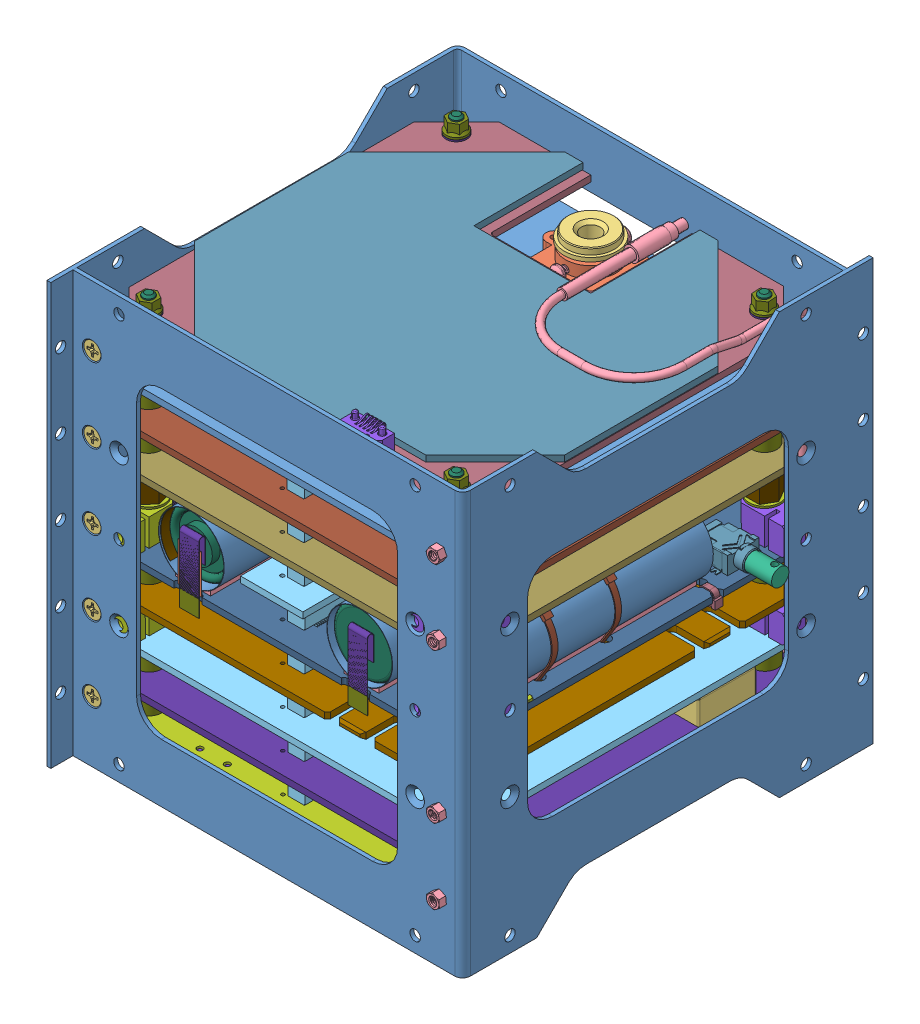
SolidWorks assembly FOX_FrameAssembly, configuration Default. Lengths in mm. (continued)
Components (placement in the parent): (continued)
- PCB-Stack-1: PCB-Stack [Default] at (24.8941 -34.8331 -20.5973) x (1 0 0) z (0 0.999997 0.002368) size (103.5 98 104.43) (continued)
  - PCB-Stack.iam-1: PCB-Stack.iam [Default] at origin size (103.5 98 104.43) (continued)
    - PCB_Exp4.iam-1: PCB_Exp4.iam [Default] at (0 0 87.6375) size (95 95 12.37) (continued)
      - Tant_Exp4_top.ipt-1: Tant_Exp4_top.ipt [Default] at (0 0 2.5749) size (95 95 1.57)
    - threaded_rod.ipt-1: threaded_rod.ipt [Default] at (-39.5 -39.5 44.6125) size (2.84 2.84 98)
    - threaded_rod.ipt-2: threaded_rod.ipt [Default] at (-39.5 39.5 44.6125) size (2.84 2.84 98)
    - threaded_rod.ipt-3: threaded_rod.ipt [Default] at (39.5 -39.5 44.6125) size (2.84 2.84 98)
    - threaded_rod.ipt-4: threaded_rod.ipt [Default] at (39.5 39.5 44.6125) size (2.84 2.84 98)
    - MS21043-04.ipt-1: MS21043-04.ipt [Default] at (-39.5 -39.5 -0.4064) x (1 0 0) z (0 0 -1) size (5.23 5.23 3.17)
    - MS21043-04.ipt-2: MS21043-04.ipt [Default] at (-39.5 39.5 -0.4064) x (1 0 0) z (0 0 -1) size (5.23 5.23 3.17)
    - MS21043-04.ipt-3: MS21043-04.ipt [Default] at (39.5 39.5 -0.4064) x (1 0 0) z (0 0 -1) size (5.23 5.23 3.17)
    - MS21043-04.ipt-4: MS21043-04.ipt [Default] at (39.5 -39.5 -0.4064) x (1 0 0) z (0 0 -1) size (5.23 5.23 3.17)
    - MS21043-04.ipt-5: MS21043-04.ipt [Default] at (-39.5 -39.5 89.6314) size (5.23 5.23 3.17)
    - MS21043-04.ipt-6: MS21043-04.ipt [Default] at (-39.5 39.5 89.6314) size (5.23 5.23 3.17)
    - MS21043-04.ipt-7: MS21043-04.ipt [Default] at (39.5 39.5 89.6314) x (0.997878 0.065108 0) z (0 0 1) size (5.23 5.23 3.17)
    - MS21043-04.ipt-8: MS21043-04.ipt [Default] at (39.5 -39.5 89.6314) size (5.23 5.23 3.17)
    - NAS620-4L.ipt-1: NAS620-4L.ipt [Default] at (-39.5 -39.5 -0.2032) x (1 0 0) z (0 0 -1) size (5.31 5.31 0.41)
    - NAS620-4L.ipt-2: NAS620-4L.ipt [Default] at (-39.5 39.5 -0.2032) x (1 0 0) z (0 0 -1) size (5.31 5.31 0.41)
    - NAS620-4L.ipt-3: NAS620-4L.ipt [Default] at (39.5 39.5 -0.2032) x (1 0 0) z (0 0 -1) size (5.31 5.31 0.41)
    - NAS620-4L.ipt-4: NAS620-4L.ipt [Default] at (39.5 -39.5 -0.2032) x (1 0 0) z (0 0 -1) size (5.31 5.31 0.41)
    - NAS620-4L.ipt-5: NAS620-4L.ipt [Default] at (-39.5 -39.5 89.4282) x (1 0 0) z (0 0 -1) size (5.31 5.31 0.41)
    - NAS620-4L.ipt-6: NAS620-4L.ipt [Default] at (-39.5 39.5 89.4282) x (0.942825 0.333287 0) z (0 0 -1) size (5.31 5.31 0.41)
    - NAS620-4L.ipt-7: NAS620-4L.ipt [Default] at (39.5 -39.5 89.4282) x (0.999994 -0.003425 0) z (0 0 -1) size (5.31 5.31 0.41)
    - NAS620-4L.ipt-8: NAS620-4L.ipt [Default] at (39.5 39.5 89.4282) x (0.997878 0.065108 0) z (0 0 1) size (5.31 5.31 0.41)
    - spacer_threaded.ipt-1: spacer_threaded.ipt [Default] at (-39.5 -39.5 58.4375) x (-0.69952 -0.714613 0) z (0 0 -1) size (7.33 6.35 9.75)
    - spacer_threaded.ipt-2: spacer_threaded.ipt [Default] at (-39.5 39.5 58.4375) x (1 0 0) z (0 0 -1) size (7.33 6.35 9.75)
    - spacer_threaded.ipt-3: spacer_threaded.ipt [Default] at (39.5 39.5 58.4375) x (1 0 0) z (0 0 -1) size (7.33 6.35 9.75)
    - spacer_threaded.ipt-4: spacer_threaded.ipt [Default] at (39.5 -39.5 58.4375) x (1 0 0) z (0 0 -1) size (7.33 6.35 9.75)
    - PCB_Exp3.iam-1: PCB_Exp3.iam [Default] at (0 0 77.9) size (95 95 15.56)
      - Samtec_QSH-030-01-L-D-A.ipt-1: Samtec_QSH-030-01-L-D-A.ipt [Default] at (0 -31.9936 -0.127) x (0 -1 0) z (1 0 0) size (21.31 4 7.49)
      - Samtec_QTH-030-02-L-D-A.ipt-1: Samtec_QTH-030-02-L-D-A.ipt [Default] at (0 -31.9938 1.8415) x (0 1 0) z (1 0 0) size (20 8 7.11)
      - PCB_Exp3.ipt-1: PCB_Exp3.ipt [Default] at origin size (95 95 1.59)
      - cameramount2.ipt-1: cameramount2.ipt [Default] at (-0.0016 34.4901 1.5875) x (0 -1 0) z (-1 0 0) size (15 7.2 23.27)
      - lens.ipt-1: lens.ipt [Default] at (-0.0016 34.4901 9.7875) size (13.5 13.5 6.5)
      - 91772A065_1-72x3-16_pan.ipt-1: 91772A065_1-72x3-16_pan.ipt [Default] at (9.4976 34.4901 4.7625) x (1 0 0) z (0 0 -1) size (3.61 3.61 6.06)
      - 91772A065_1-72x3-16_pan.ipt-2: 91772A065_1-72x3-16_pan.ipt [Default] at (-9.5016 34.4901 4.7625) x (1 0 0) z (0 0 -1) size (3.61 3.61 6.06)
      - 91772A065_1-72x3-16_pan.ipt-3: 91772A065_1-72x3-16_pan.ipt [Default] at (-0.0016 37.7276 6.7875) x (1 0 0) z (0 1 0) size (3.61 3.61 6.06)
      - 91772A065_1-72x3-16_pan.ipt-4: 91772A065_1-72x3-16_pan.ipt [Default] at (-0.0016 31.2526 6.7875) x (-0.84925 0 0.527992) z (0 -1 0) size (3.61 3.61 6.06)
    - PCB_Batt2.iam-1: PCB_Batt2.iam [Default] at (0 0 48.6875) size (16 31 12.08)
      - PCB_Batt2.ipt-1: PCB_Batt2.ipt [Default] at origin size (16 31 1.59)
      - Samtec_QTH-030-02-L-D-A.ipt-1: Samtec_QTH-030-02-L-D-A.ipt [Default] at (0 -31.9938 1.8415) x (0 1 0) z (1 0 0) size (20 8 7.11)
      - Samtec_QSH-030-01-L-D-A.ipt-1: Samtec_QSH-030-01-L-D-A.ipt [Default] at (0 -31.9936 -0.127) x (0 -1 0) z (1 0 0) size (21.31 4 7.49)
    - safe_rbf.ipt-1: safe_rbf.ipt [Default] at (36.5 28.5 43.1175) size (18 4.45 4.46)
    - delrin_pcb_mount4_magnet.ipt-1: delrin_pcb_mount4_magnet.ipt [Default] at (-49 -49 25.1375) size (14 14 7)
    - delrin_pcb_mount4_magnet.ipt-2: delrin_pcb_mount4_magnet.ipt [Default] at (-49 -49 44.6125) x (0 1 0) z (0 0 -1) size (14 14 7)
    - magnet.iam-1: magnet.iam [Default] at (-44.5 -44.5 38.2125) size (6.35 6.35 51.8)
      - magnet.ipt-1: magnet.ipt [Default] at origin size (3.17 3.17 51.8)
      - magnet_spacer.ipt-1: magnet_spacer.ipt [Default] at (0 0 -3.33) size (6.35 6.35 23)
Mates (geometry in assembly coordinates):
- Coincident1: coincident: plane of FOX_ME_111_Walls-1 through (105.9061 -40.5308 28.0204) normal (0 0 -1); plane of FOX_ME_111_Walls-2 through (-55.1289 -40.5308 -70.6584) normal (0 0 -1)
- Concentric1: concentric: circle of FOX_ME_111_Walls-1; circle of FOX_ME_111_Walls-2
- Coincident2: coincident: plane of FOX_ME_111_Walls-1 through (105.9061 -40.5308 29.0204) normal (0 0 1); plane of FOX_ME_111_Walls-2 through (-55.1289 -40.5308 -69.6584) normal (0 0 1)
- Concentric2: concentric: circle of FOX_ME_111_Walls-1; circle of FOX_ME_111_Walls-2
- Concentric3: concentric: circle of FOX_ME_111_Walls-2; circle of 93085A017_Mil. Spec. Stainless Steel Phillips Flat Head Screws-10
- Concentric4: concentric: circle of FOX_ME_111_Walls-2; circle of 93085A017_Mil. Spec. Stainless Steel Phillips Flat Head Screws-9
- Concentric5: concentric: circle of FOX_ME_111_Walls-2; circle of 93085A017_Mil. Spec. Stainless Steel Phillips Flat Head Screws-8
- Concentric6: concentric: circle of FOX_ME_111_Walls-2; circle of 93085A017_Mil. Spec. Stainless Steel Phillips Flat Head Screws-7
- Concentric7: concentric: circle of FOX_ME_111_Walls-2; circle of 93085A017_Mil. Spec. Stainless Steel Phillips Flat Head Screws-6
- Concentric8: concentric anti-aligned: circle of FOX_ME_111_Walls-1; circle of 93085A017_Mil. Spec. Stainless Steel Phillips Flat Head Screws-2
- Concentric9: concentric: circle of FOX_ME_111_Walls-1; circle of 93085A017_Mil. Spec. Stainless Steel Phillips Flat Head Screws-5
- Concentric10: concentric: circle of FOX_ME_111_Walls-1; circle of 93085A017_Mil. Spec. Stainless Steel Phillips Flat Head Screws-1
- Concentric11: concentric: circle of FOX_ME_111_Walls-1; circle of 93085A017_Mil. Spec. Stainless Steel Phillips Flat Head Screws-3
- Concentric12: concentric: circle of FOX_ME_111_Walls-1; circle of 93085A017_Mil. Spec. Stainless Steel Phillips Flat Head Screws-4
- Coincident3: coincident: cone of FOX_ME_111_Walls-2 through (70.0611 48.2692 -70.6584) axis (0 0 1); cone of 93085A017_Mil. Spec. Stainless Steel Phillips Flat Head Screws-10 through (70.0611 48.2692 -69.5611) axis (0 0 1)
- Coincident4: coincident: cone of FOX_ME_111_Walls-2 through (70.0611 29.0692 -70.6584) axis (0 0 1); cone of 93085A017_Mil. Spec. Stainless Steel Phillips Flat Head Screws-9 through (70.0611 29.0692 -69.5611) axis (0 0 1)
- Coincident5: coincident: cone of FOX_ME_111_Walls-2 through (70.0611 9.8692 -70.6584) axis (0 0 1); cone of 93085A017_Mil. Spec. Stainless Steel Phillips Flat Head Screws-8 through (70.0611 9.8692 -69.5611) axis (0 0 1)
- Coincident6: coincident: cone of FOX_ME_111_Walls-2 through (70.0611 -9.3308 -70.6584) axis (0 0 1); cone of 93085A017_Mil. Spec. Stainless Steel Phillips Flat Head Screws-7 through (70.0611 -9.3308 -69.5611) axis (0 0 1)
- Coincident7: coincident: cone of FOX_ME_111_Walls-2 through (70.0611 -28.5308 -70.6584) axis (0 0 1); cone of 93085A017_Mil. Spec. Stainless Steel Phillips Flat Head Screws-6 through (70.0611 -28.5308 -69.5611) axis (0 0 1)
- Coincident8: coincident: cone of FOX_ME_111_Walls-1 through (-19.2839 48.2692 29.0204) axis (0 0 -1); cone of 93085A017_Mil. Spec. Stainless Steel Phillips Flat Head Screws-2 through (-19.2839 48.2692 27.923) axis (0 0 -1)
- Coincident9: coincident: cone of FOX_ME_111_Walls-1 through (-19.2839 29.0692 29.0204) axis (0 0 -1); cone of 93085A017_Mil. Spec. Stainless Steel Phillips Flat Head Screws-5 through (-19.2839 29.0692 27.923) axis (0 0 -1)
- Coincident10: coincident: cone of FOX_ME_111_Walls-1 through (-19.2839 9.8692 29.0204) axis (0 0 -1); cone of 93085A017_Mil. Spec. Stainless Steel Phillips Flat Head Screws-1 through (-19.2839 9.8692 27.923) axis (0 0 -1)
- Coincident11: coincident: cone of FOX_ME_111_Walls-1 through (-19.2839 -28.5308 29.0204) axis (0 0 -1); cone of 93085A017_Mil. Spec. Stainless Steel Phillips Flat Head Screws-4 through (-19.2839 -28.5308 27.923) axis (0 0 -1)
- Coincident12: coincident: cone of FOX_ME_111_Walls-1 through (-19.2839 -9.3308 29.0204) axis (0 0 -1); cone of 93085A017_Mil. Spec. Stainless Steel Phillips Flat Head Screws-3 through (-19.2839 -9.3308 27.923) axis (0 0 -1)
- Concentric13: concentric: circle of 90945A705_18-8 Stainless Steel Mil. Spec. Washer-9; circle of FOX_ME_111_Walls-1
- Coincident13: coincident: plane of FOX_ME_111_Walls-1 through (105.9061 -40.5308 28.0204) normal (0 0 -1); plane of 90945A705_18-8 Stainless Steel Mil. Spec. Washer-9 through (70.0611 29.0692 28.0204) normal (0 0 -1)
- Concentric14: concentric: circle of FOX_ME_111_Walls-1; circle of 90945A705_18-8 Stainless Steel Mil. Spec. Washer-8
- Coincident15: coincident: plane of FOX_ME_111_Walls-1 through (105.9061 -40.5308 28.0204) normal (0 0 -1); plane of 90945A705_18-8 Stainless Steel Mil. Spec. Washer-8 through (70.0611 48.2692 28.0204) normal (0 0 -1)
- Concentric15: concentric: circle of FOX_ME_111_Walls-1; circle of 90945A705_18-8 Stainless Steel Mil. Spec. Washer-5
- Coincident17: coincident: plane of FOX_ME_111_Walls-1 through (105.9061 -40.5308 28.0204) normal (0 0 -1); plane of 90945A705_18-8 Stainless Steel Mil. Spec. Washer-7 through (70.0611 -9.3308 28.0204) normal (0 0 -1)
- Concentric16: concentric: circle of FOX_ME_111_Walls-1; circle of 90945A705_18-8 Stainless Steel Mil. Spec. Washer-7
- Coincident18: coincident: plane of FOX_ME_111_Walls-1 through (105.9061 -40.5308 28.0204) normal (0 0 -1); plane of 90945A705_18-8 Stainless Steel Mil. Spec. Washer-1 through (70.0611 -28.5308 28.0204) normal (0 0 -1)
- Concentric17: concentric: circle of FOX_ME_111_Walls-1; circle of 90945A705_18-8 Stainless Steel Mil. Spec. Washer-1
- Coincident19: coincident: plane of FOX_ME_111_Walls-2 through (-55.1289 -40.5308 -69.6584) normal (0 0 1); plane of 90945A705_18-8 Stainless Steel Mil. Spec. Washer-2 through (-19.2839 -28.5308 -69.6584) normal (0 0 1)
- Concentric18: concentric: circle of FOX_ME_111_Walls-2; circle of 90945A705_18-8 Stainless Steel Mil. Spec. Washer-2
- Coincident20: coincident: plane of FOX_ME_111_Walls-2 through (-55.1289 -40.5308 -69.6584) normal (0 0 1); plane of 90945A705_18-8 Stainless Steel Mil. Spec. Washer-4 through (-19.2839 -9.3308 -69.6584) normal (0 0 1)
- Concentric19: concentric: circle of FOX_ME_111_Walls-2; circle of 90945A705_18-8 Stainless Steel Mil. Spec. Washer-4
- Coincident21: coincident: plane of FOX_ME_111_Walls-2 through (-55.1289 -40.5308 -69.6584) normal (0 0 1); plane of 90945A705_18-8 Stainless Steel Mil. Spec. Washer-6 through (-19.2839 9.8692 -69.6584) normal (0 0 1)
- Concentric20: concentric: circle of FOX_ME_111_Walls-2; circle of 90945A705_18-8 Stainless Steel Mil. Spec. Washer-6
- Coincident22: coincident: plane of FOX_ME_111_Walls-2 through (-55.1289 -40.5308 -69.6584) normal (0 0 1); plane of 90945A705_18-8 Stainless Steel Mil. Spec. Washer-3 through (-19.2839 29.0692 -69.6584) normal (0 0 1)
- Concentric21: concentric: circle of FOX_ME_111_Walls-2; circle of 90945A705_18-8 Stainless Steel Mil. Spec. Washer-3
- Concentric33: concentric: circle of 90945A705_18-8 Stainless Steel Mil. Spec. Washer-7; circle of 95307A800_Mil. Spec. Distorted-Thread Flange Locknut-1
- Parallel1: parallel anti-aligned: plane of 93085A017_Mil. Spec. Stainless Steel Phillips Flat Head Screws-7 through (70.0611 -9.3308 -67.3025) normal (0 -1 0)
- Screw3: screw = 10: cylinder of 93085A017_Mil. Spec. Stainless Steel Phillips Flat Head Screws-7 through (70.0611 -9.3308 -64.1275) axis (0 0 1) radius 1.0922; cylinder of 95307A800_Mil. Spec. Distorted-Thread Flange Locknut-1 through (70.0611 -9.3308 28.4776) axis (0 0 1) radius 0.7976
- LimitDistance1: limit distance = 0 mm anti-aligned: plane of 90945A705_18-8 Stainless Steel Mil. Spec. Washer-7 through (70.0611 -9.3308 28.4776) normal (0 0 1); plane of 95307A800_Mil. Spec. Distorted-Thread Flange Locknut-1 through (71.509 -8.2067 28.4776) normal (0 0 -1)
- Parallel4: parallel: plane of assembly through (0 0 0) normal (1 0 0); plane of 90945A705_18-8 Stainless Steel Mil. Spec. Washer-1 through (70.0611 -28.5308 28.0204) normal (1 0 0); plane of assembly
- Parallel5: parallel: plane of assembly through (0 0 0) normal (1 0 0); plane of 90945A705_18-8 Stainless Steel Mil. Spec. Washer-2 through (-19.2839 -28.5308 -69.6584) normal (1 0 0); plane of assembly
- Parallel7: parallel aligned: plane of 93085A017_Mil. Spec. Stainless Steel Phillips Flat Head Screws-1 through (-19.2839 9.8692 25.6645) normal (0 1 0)
- Parallel8: parallel: plane of assembly through (0 0 0) normal (1 0 0); plane of 93085A017_Mil. Spec. Stainless Steel Phillips Flat Head Screws-10 through (70.0611 48.2692 -67.3025) normal (-1 0 0); plane of assembly
- Parallel9: parallel anti-aligned: plane of 93085A017_Mil. Spec. Stainless Steel Phillips Flat Head Screws-9 through (70.0611 29.0692 -67.3025) normal (0 -1 0)
- Parallel10: parallel: plane of assembly through (0 0 0) normal (1 0 0); plane of 93085A017_Mil. Spec. Stainless Steel Phillips Flat Head Screws-8 through (70.0611 9.8692 -67.3025) normal (1 0 0); plane of assembly
- Parallel11: parallel: plane of assembly through (0 0 0) normal (1 0 0); plane of 93085A017_Mil. Spec. Stainless Steel Phillips Flat Head Screws-6 through (70.0611 -28.5308 -67.3025) normal (1 0 0); plane of assembly
- Parallel12: parallel: plane of assembly through (0 0 0) normal (1 0 0); plane of 93085A017_Mil. Spec. Stainless Steel Phillips Flat Head Screws-5 through (-19.2839 29.0692 25.6645) normal (1 0 0); plane of assembly
- Parallel13: parallel: plane of assembly through (0 0 0) normal (1 0 0); plane of 93085A017_Mil. Spec. Stainless Steel Phillips Flat Head Screws-2 through (-19.2839 48.2692 25.6645) normal (1 0 0); plane of assembly
- Parallel14: parallel: plane of assembly through (0 0 0) normal (1 0 0); plane of 93085A017_Mil. Spec. Stainless Steel Phillips Flat Head Screws-3 through (-19.2839 -9.3308 25.6645) normal (1 0 0); plane of assembly
- Parallel15: parallel: plane of assembly through (0 0 0) normal (1 0 0); plane of 93085A017_Mil. Spec. Stainless Steel Phillips Flat Head Screws-4 through (-19.2839 -28.5308 25.6645) normal (1 0 0); plane of assembly
- Concentric34: concentric: circle of 93085A017_Mil. Spec. Stainless Steel Phillips Flat Head Screws-2; circle of 90945A705_18-8 Stainless Steel Mil. Spec. Washer-20
- Coincident41: coincident: plane of FOX_ME_111_Walls-2 through (-55.1289 -40.5308 -69.6584) normal (0 0 1); plane of 90945A705_18-8 Stainless Steel Mil. Spec. Washer-20 through (-19.2839 48.2692 -69.6584) normal (0 0 1)
- Parallel16: parallel: plane of assembly through (0 0 0) normal (1 0 0); plane of 90945A705_18-8 Stainless Steel Mil. Spec. Washer-3 through (-19.2839 29.0692 -69.6584) normal (1 0 0); plane of assembly
- Parallel17: parallel: plane of assembly through (0 0 0) normal (1 0 0); plane of 90945A705_18-8 Stainless Steel Mil. Spec. Washer-4 through (-19.2839 -9.3308 -69.6584) normal (1 0 0); plane of assembly
- Parallel18: parallel: plane of assembly through (0 0 0) normal (1 0 0); plane of 90945A705_18-8 Stainless Steel Mil. Spec. Washer-5 through (70.0611 9.8692 -68.6584) normal (1 0 0); plane of assembly
- Parallel19: parallel: plane of assembly through (0 0 0) normal (1 0 0); plane of 90945A705_18-8 Stainless Steel Mil. Spec. Washer-6 through (-19.2839 9.8692 -69.6584) normal (1 0 0); plane of assembly
- Parallel20: parallel: plane of assembly through (0 0 0) normal (1 0 0); plane of 90945A705_18-8 Stainless Steel Mil. Spec. Washer-7 through (70.0611 -9.3308 28.0204) normal (1 0 0); plane of assembly
- Parallel21: parallel: plane of assembly through (0 0 0) normal (1 0 0); plane of 90945A705_18-8 Stainless Steel Mil. Spec. Washer-8 through (70.0611 48.2692 28.0204) normal (1 0 0); plane of assembly
- Parallel22: parallel: plane of assembly through (0 0 0) normal (1 0 0); plane of 90945A705_18-8 Stainless Steel Mil. Spec. Washer-9 through (70.0611 29.0692 28.0204) normal (1 0 0); plane of assembly
- Parallel23: parallel: plane of assembly through (0 0 0) normal (1 0 0); plane of 90945A705_18-8 Stainless Steel Mil. Spec. Washer-20 through (-19.2839 48.2692 -70.1156) normal (1 0 0); plane of assembly
- Concentric36: concentric: circle of 90945A705_18-8 Stainless Steel Mil. Spec. Washer-20; circle of 95307A800_Mil. Spec. Distorted-Thread Flange Locknut-6
- Concentric37: concentric: circle of 90945A705_18-8 Stainless Steel Mil. Spec. Washer-3; circle of 95307A800_Mil. Spec. Distorted-Thread Flange Locknut-7
- Concentric38: concentric: circle of 90945A705_18-8 Stainless Steel Mil. Spec. Washer-6; circle of 95307A800_Mil. Spec. Distorted-Thread Flange Locknut-8
- Concentric39: concentric: circle of 90945A705_18-8 Stainless Steel Mil. Spec. Washer-4; circle of 95307A800_Mil. Spec. Distorted-Thread Flange Locknut-9
- Concentric40: concentric: circle of 90945A705_18-8 Stainless Steel Mil. Spec. Washer-2; circle of 95307A800_Mil. Spec. Distorted-Thread Flange Locknut-10
- Concentric41: concentric: circle of 90945A705_18-8 Stainless Steel Mil. Spec. Washer-8; circle of 95307A800_Mil. Spec. Distorted-Thread Flange Locknut-2
- Concentric42: concentric: circle of 90945A705_18-8 Stainless Steel Mil. Spec. Washer-9; circle of 95307A800_Mil. Spec. Distorted-Thread Flange Locknut-3
- Concentric43: concentric: circle of 90945A705_18-8 Stainless Steel Mil. Spec. Washer-5; circle of 95307A800_Mil. Spec. Distorted-Thread Flange Locknut-4
- Concentric44: concentric: circle of 90945A705_18-8 Stainless Steel Mil. Spec. Washer-1; circle of 95307A800_Mil. Spec. Distorted-Thread Flange Locknut-5
- Screw4: screw = 10 aligned: cylinder of 93085A017_Mil. Spec. Stainless Steel Phillips Flat Head Screws-2 through (-19.2839 48.2692 22.4895) axis (0 0 -1) radius 1.0922; cylinder of 95307A800_Mil. Spec. Distorted-Thread Flange Locknut-6 through (-19.2839 48.2692 -70.1156) axis (0 0 -1) radius 0.7976
- LimitDistance2: limit distance = 0 mm anti-aligned: plane of 95307A800_Mil. Spec. Distorted-Thread Flange Locknut-6 through (-21.1104 48.425 -70.1156) normal (0 0 1); plane of 90945A705_18-8 Stainless Steel Mil. Spec. Washer-20 through (-19.2839 48.2692 -70.1156) normal (0 0 -1)
- Screw5: screw = 10: cylinder of 93085A017_Mil. Spec. Stainless Steel Phillips Flat Head Screws-5 through (-19.2839 29.0692 22.4895) axis (0 0 -1) radius 1.0922; cylinder of 95307A800_Mil. Spec. Distorted-Thread Flange Locknut-7 through (-19.2839 29.0692 -70.1156) axis (0 0 -1) radius 0.7976
- LimitDistance3: limit distance = 0 mm anti-aligned: plane of 95307A800_Mil. Spec. Distorted-Thread Flange Locknut-7 through (-18.7119 27.3277 -70.1156) normal (0 0 1); plane of 90945A705_18-8 Stainless Steel Mil. Spec. Washer-3 through (-19.2839 29.0692 -70.1156) normal (0 0 -1)
- Screw6: screw = 10: cylinder of 93085A017_Mil. Spec. Stainless Steel Phillips Flat Head Screws-1 through (-19.2839 9.8692 22.4895) axis (0 0 -1) radius 1.0922; cylinder of 95307A800_Mil. Spec. Distorted-Thread Flange Locknut-8 through (-19.2839 9.8692 -70.1156) axis (0 0 -1) radius 0.7976
- LimitDistance4: limit distance = 0 mm anti-aligned: plane of 95307A800_Mil. Spec. Distorted-Thread Flange Locknut-8 through (-18.1017 8.4683 -70.1156) normal (0 0 1); plane of 90945A705_18-8 Stainless Steel Mil. Spec. Washer-6 through (-19.2839 9.8692 -70.1156) normal (0 0 -1)
- Screw8: screw = 10: cylinder of 93085A017_Mil. Spec. Stainless Steel Phillips Flat Head Screws-3 through (-19.2839 -9.3308 22.4895) axis (0 0 -1) radius 1.0922; cylinder of 95307A800_Mil. Spec. Distorted-Thread Flange Locknut-9 through (-19.2839 -9.3308 -70.1156) axis (0 0 -1) radius 0.7976
- LimitDistance5: limit distance = 0 mm anti-aligned: plane of 95307A800_Mil. Spec. Distorted-Thread Flange Locknut-9 through (-20.9202 -8.5044 -70.1156) normal (0 0 1); plane of 90945A705_18-8 Stainless Steel Mil. Spec. Washer-4 through (-19.2839 -9.3308 -70.1156) normal (0 0 -1)
- Screw10: screw = 10: cylinder of 93085A017_Mil. Spec. Stainless Steel Phillips Flat Head Screws-4 through (-19.2839 -28.5308 22.4895) axis (0 0 -1) radius 1.0922; cylinder of 95307A800_Mil. Spec. Distorted-Thread Flange Locknut-10 through (-19.2839 -28.5308 -70.1156) axis (0 0 -1) radius 0.7976
- LimitDistance6: limit distance = 0 mm anti-aligned: plane of 95307A800_Mil. Spec. Distorted-Thread Flange Locknut-10 through (-17.8562 -27.3812 -70.1156) normal (0 0 1); plane of 90945A705_18-8 Stainless Steel Mil. Spec. Washer-2 through (-19.2839 -28.5308 -70.1156) normal (0 0 -1)
- Screw11: screw = 10: cylinder of 93085A017_Mil. Spec. Stainless Steel Phillips Flat Head Screws-6 through (70.0611 -28.5308 -64.1275) axis (0 0 1) radius 1.0922; cylinder of 95307A800_Mil. Spec. Distorted-Thread Flange Locknut-5 through (70.0611 -28.5308 28.4776) axis (0 0 1) radius 0.7976
- LimitDistance7: limit distance = 0 mm anti-aligned: plane of 95307A800_Mil. Spec. Distorted-Thread Flange Locknut-5 through (71.7324 -29.2836 28.4776) normal (0 0 -1); plane of 90945A705_18-8 Stainless Steel Mil. Spec. Washer-1 through (70.0611 -28.5308 28.4776) normal (0 0 1)
- Screw12: screw = 10: cylinder of 93085A017_Mil. Spec. Stainless Steel Phillips Flat Head Screws-8 through (70.0611 9.8692 -64.1275) axis (0 0 1) radius 1.0922; cylinder of 95307A800_Mil. Spec. Distorted-Thread Flange Locknut-4 through (70.0611 9.8692 -68.2012) axis (0 0 1) radius 0.7976
- LimitDistance8: limit distance = 0 mm anti-aligned: plane of 95307A800_Mil. Spec. Distorted-Thread Flange Locknut-4 through (68.2284 9.8293 -68.2012) normal (0 0 -1); plane of 90945A705_18-8 Stainless Steel Mil. Spec. Washer-5 through (70.0611 9.8692 -68.2012) normal (0 0 1)
- Screw14: screw = 10: cylinder of 93085A017_Mil. Spec. Stainless Steel Phillips Flat Head Screws-9 through (70.0611 29.0692 -64.1275) axis (0 0 1) radius 1.0922; cylinder of 95307A800_Mil. Spec. Distorted-Thread Flange Locknut-3 through (70.0611 29.0692 28.4776) axis (0 0 1) radius 0.7976
- LimitDistance9: limit distance = 0 mm anti-aligned: plane of 95307A800_Mil. Spec. Distorted-Thread Flange Locknut-3 through (70.1322 27.2375 28.4776) normal (0 0 -1); plane of 90945A705_18-8 Stainless Steel Mil. Spec. Washer-9 through (70.0611 29.0692 28.4776) normal (0 0 1)
- Screw15: screw = 10: cylinder of 93085A017_Mil. Spec. Stainless Steel Phillips Flat Head Screws-10 through (70.0611 48.2692 -64.1275) axis (0 0 1) radius 1.0922; cylinder of 95307A800_Mil. Spec. Distorted-Thread Flange Locknut-2 through (70.0611 48.2692 28.4776) axis (0 0 1) radius 0.7976
- LimitDistance10: limit distance = 0 mm anti-aligned: plane of 95307A800_Mil. Spec. Distorted-Thread Flange Locknut-2 through (69.2389 49.9076 28.4776) normal (0 0 -1); plane of 90945A705_18-8 Stainless Steel Mil. Spec. Washer-8 through (70.0611 48.2692 28.4776) normal (0 0 1)
- Coincident44: coincident anti-aligned: plane of FOX_ME_111_Walls-2 through (-24.1059 -40.5308 -38.9915) normal (1 0 0); plane of PCB-Stack-1/PCB-Stack.iam-1/delrin_pcb_mount4_magnet.ipt-1 through (-24.1059 -9.8117 28.4621) normal (-1 0 0)
- Concentric54: concentric anti-aligned: circle of FOX_ME_111_Walls-2; circle of PCB-Stack-1/PCB-Stack.iam-1/delrin_pcb_mount4.ipt-2
